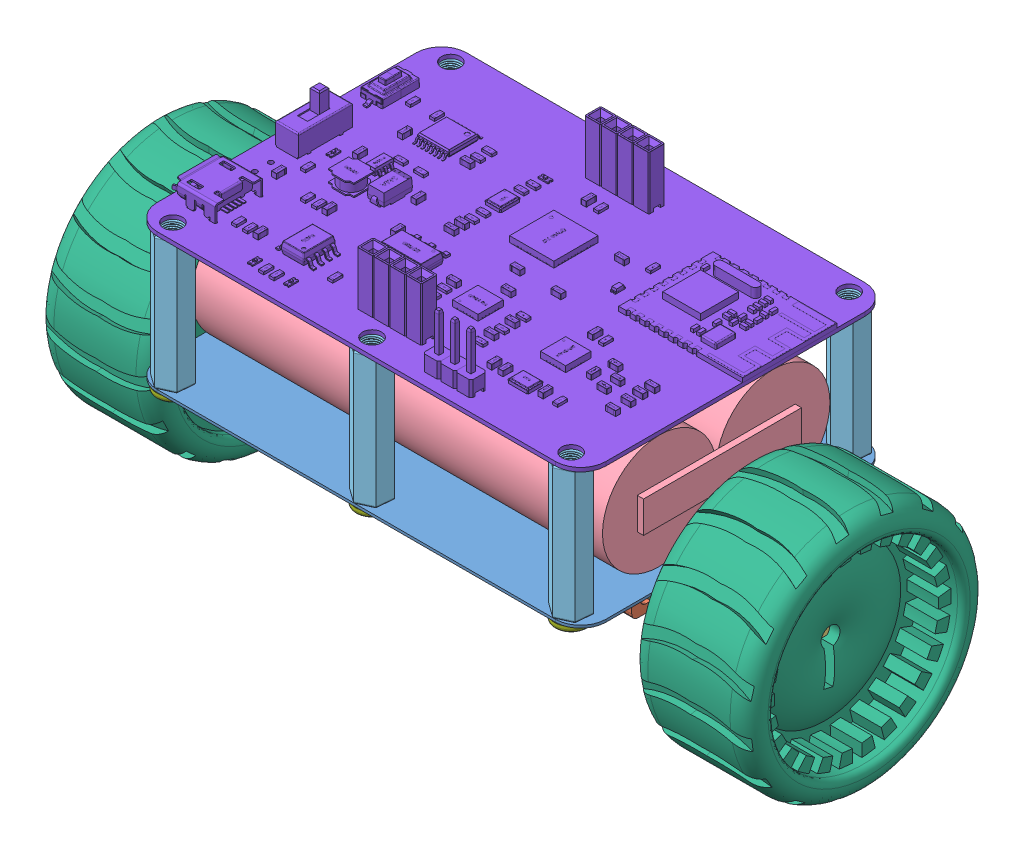
SolidWorks assembly 平衡小车装配体, configuration Default. Lengths in mm.
Overall size (112.99 59.89 50.48).
21 component instances, 8 part files, 29 mates.
Components (placement in the parent):
- 底盘-1: 底盘 [Default] at (53.4104 0 22.4882) x (1 0 -0.000387) z (0 1 0) size (71 49 0.41)
- N20电机座-1: N20电机座 [Default] at (68.1983 -0.4115 22.4825) x (1 0 -0.000387) z (-0.000387 0 -1) size (11.5 11.15 26)
- 电机-1: 电机 [Default] at (68.1983 -5.2615 22.3325) x (0.000387 0 1) z (1 0 -0.000387) size (12.1 14.5 40.5)
- 锂电池-1: 锂电池 [Default] at (20.9104 9 22.5453) x (0.000387 0 1) z (0 1 0) size (36 67 18)
- N20电机座-2: N20电机座 [Default] at (38.6224 -0.4115 22.4939) x (-1 0 0.000387) z (0.000387 0 1) size (11.5 11.15 26)
- 电机-2: 电机 [Default] at (38.6223 -5.2615 22.3439) x (-0.000387 0 -1) z (-1 0 0.000387) size (12.1 14.5 40.5)
- 铜柱M3x21-1: 铜柱M3x21 [Default] at (21.9189 0 44.5004) x (0.910173 0 -0.414228) z (0.414228 0 0.910173) size (5.37 21 4.65)
- 轮子φ43-1: 轮子φ43 [Default] at (100.3983 -5.2615 22.32) x (0.00009 -0.972822 0.231553) z (-0.000376 -0.231553 -0.972822) size (38.37 19 38.37)
- 轮子φ43-2: 轮子φ43 [Default] at (6.4223 -5.2615 22.3564) x (0.00013 -0.942269 0.334857) z (0.000365 0.334857 0.942269) size (38.37 19 38.37)
- 铜柱M3x21-9: 铜柱M3x21 [Default] at (21.9019 0 0.5004) x (0.910173 0 -0.414228) z (0.414228 0 0.910173) size (5.37 21 4.65)
- 铜柱M3x21-10: 铜柱M3x21 [Default] at (53.4189 0 44.4882) x (0.910173 0 -0.414228) z (0.414228 0 0.910173) size (5.37 21 4.65)
- 铜柱M3x21-11: 铜柱M3x21 [Default] at (53.4019 0 0.4882) x (0.910173 0 -0.414228) z (0.414228 0 0.910173) size (5.37 21 4.65)
- 铜柱M3x21-12: 铜柱M3x21 [Default] at (84.9189 0 44.476) x (0.910173 0 -0.414228) z (0.414228 0 0.910173) size (5.37 21 4.65)
- 铜柱M3x21-13: 铜柱M3x21 [Default] at (84.9019 0 0.476) x (0.910173 0 -0.414228) z (0.414228 0 0.910173) size (5.37 21 4.65)
- 螺丝钉M3x6-1: 螺丝钉M3x6 [Default] at (21.9189 -0.4115 44.5004) x (0 1 0) z (0 0 1) size (7.68 5.2 5.2)
- 螺丝钉M3x6-2: 螺丝钉M3x6 [Default] at (21.9019 -0.4115 0.5004) x (0 1 0) z (0 0 1) size (7.68 5.2 5.2)
- 螺丝钉M3x6-3: 螺丝钉M3x6 [Default] at (53.4189 -0.4115 44.4882) x (0 1 0) z (0 0 1) size (7.68 5.2 5.2)
- 螺丝钉M3x6-4: 螺丝钉M3x6 [Default] at (53.4019 -0.4115 0.4882) x (0 1 0) z (0 0 1) size (7.68 5.2 5.2)
- 螺丝钉M3x6-5: 螺丝钉M3x6 [Default] at (84.9189 -0.4115 44.476) x (0 1 0) z (0 0 1) size (7.68 5.2 5.2)
- 螺丝钉M3x6-6: 螺丝钉M3x6 [Default] at (84.9019 -0.4115 0.476) x (0 1 0) z (0 0 1) size (7.68 5.2 5.2)
- 平衡小车主板-1: 平衡小车主板 [Default] at (53.4104 21.6237 22.4882) x (1 0 -0.000387) z (0 1 0) size (71.11 49 13.51)
Mates (geometry in assembly coordinates):
- 重合8: coincident anti-aligned: plane of N20电机座-1 through (79.7006 -0.4115 28.378) normal (-0.000387 0 -1); plane of 电机-1 through (83.2006 -0.2615 28.3767) normal (0.000387 0 1)
- 重合12: coincident anti-aligned: plane of N20电机座-2 through (27.1247 -10.2615 28.3984) normal (-0.000387 0 -1); plane of 电机-2 through (23.6247 -0.2615 28.3997) normal (0.000387 0 1)
- 重合13: coincident anti-aligned: plane of N20电机座-2 through (38.6224 -0.4115 22.4939) normal (1 0 -0.000387); plane of 电机-2 through (38.6223 -5.2615 22.3439) normal (-1 0 0.000387)
- 重合15: coincident aligned: plane of 底盘-1 through (17.9958 0 41.5879) normal (0 1 0)
- 重合17: coincident anti-aligned: plane of 底盘-1 through (22.9017 -0.4115 0) normal (0 0 -1)
- 重合19: coincident anti-aligned: circle of 电机-1; plane of 轮子φ43-1 through (92.8996 -19.8538 25.7962) normal (-1 0 0.000387)
- 同心7: concentric aligned: cylinder of 电机-1 through (102.1983 -5.2615 22.3193) axis (-1 0 0.000387) radius 1.5; cylinder of 轮子φ43-1 through (107.8983 -5.2615 22.3171) axis (-1 0 0.000387) radius 1.5
- 重合20: coincident anti-aligned: plane of 电机-2 through (13.9223 -5.2615 22.3535) normal (-1 0 0.000387); plane of 轮子φ43-2 through (13.9243 -19.3955 27.3763) normal (1 0 -0.000387)
- 同心8: concentric aligned: cylinder of 电机-2 through (4.6223 -5.2615 22.3571) axis (1 0 -0.000387) radius 1.5; cylinder of 轮子φ43-2 through (-1.0777 -5.2615 22.3593) axis (1 0 -0.000387) radius 1.5
- 同心9: concentric anti-aligned: cylinder of N20电机座-2 through (34.407 -1.8115 13.6956) axis (0 1 0) radius 1.125; cylinder of 底盘-1 through (34.407 -0.4115 13.6956) axis (0 -1 0) radius 1.5
- 同心10: concentric anti-aligned: cylinder of 底盘-1 through (34.4138 -0.4115 31.2955) axis (0 -1 0) radius 1.5; cylinder of N20电机座-2 through (34.4138 -1.8115 31.2955) axis (0 1 0) radius 1.125
- 同心11: concentric anti-aligned: cylinder of 底盘-1 through (72.4138 -0.4115 31.2808) axis (0 -1 0) radius 1.5; cylinder of N20电机座-1 through (72.4138 -1.8115 31.2808) axis (0 1 0) radius 1.125
- 同心12: concentric anti-aligned: cylinder of 底盘-1 through (72.407 -0.4115 13.6808) axis (0 -1 0) radius 1.5; cylinder of N20电机座-1 through (72.407 -1.8115 13.6808) axis (0 1 0) radius 1.125
- 重合21: coincident aligned: cylinder of 底盘-1 through (21.9189 -0.4115 44.5004) axis (0 -1 0) radius 1.5; circle of 铜柱M3x21-1
- 重合22: coincident anti-aligned: plane of 底盘-1 through (17.9183 0 43.0149) normal (0 1 0); plane of 铜柱M3x21-1 through (21.9189 0 44.5004) normal (0 -1 0)
- 重合23: coincident anti-aligned: plane of N20电机座-1 through (79.7006 -10.2615 28.378) normal (0 1 0); plane of 电机-1 through (83.1959 -10.2615 16.2767) normal (0 -1 0)
- 重合24: coincident anti-aligned: plane of 底盘-1 through (17.9183 -0.4115 43.0149) normal (0 -1 0); plane of N20电机座-1 through (79.7006 -0.4115 28.378) normal (0 1 0)
- 重合25: coincident anti-aligned: plane of N20电机座-2 through (27.1201 -10.2615 16.5984) normal (0 1 0); plane of 电机-2 through (23.6247 -10.2615 28.3997) normal (0 -1 0)
- 重合26: coincident anti-aligned: plane of 底盘-1 through (17.9183 -0.4115 43.0149) normal (0 -1 0); plane of N20电机座-2 through (27.1201 -0.4115 16.5984) normal (0 1 0)
- 重合27: coincident anti-aligned: plane of N20电机座-1 through (68.1983 -0.4115 22.4825) normal (-1 0 0.000387); plane of 电机-1 through (68.1983 -5.2615 22.3325) normal (1 0 -0.000387)
- 平行1: parallel anti-aligned: plane of 底盘-1 through (17.9183 0 43.0149) normal (0 1 0); plane of 锂电池-1 through (86.9055 6.5 10.0198) normal (0 -1 0)
- 距离1: distance = 6.5 mm anti-aligned: plane of 锂电池-1 through (86.9055 6.5 10.0198) normal (0 -1 0); plane of 底盘-1 through (17.9183 0 43.0149) normal (0 1 0)
- 平行2: parallel aligned: plane of 底盘-1 through (84.8879 -0.4115 -2.024) normal (-0.000387 0 -1); plane of 锂电池-1 through (86.9055 11.5 10.0198) normal (-0.000387 0 -1)
- 距离2: distance = 2 mm aligned: plane of 底盘-1 through (88.9183 -0.4115 42.9875) normal (1 0 -0.000387); plane of 锂电池-1 through (86.9104 9 22.5198) normal (1 0 -0.000387)
- 重合28: coincident anti-aligned: plane of 底盘-1 through (17.9183 -0.4115 43.0149) normal (0 -1 0); plane of 螺丝钉M3x6-1 through (21.9189 -0.4115 44.5004) normal (0 1 0)
- 同心13: concentric aligned: cylinder of 底盘-1 through (21.9189 -0.4115 44.5004) axis (0 -1 0) radius 1.5; circle of 螺丝钉M3x6-1
- 重合29: coincident anti-aligned: plane of 铜柱M3x21-1 through (21.9189 21 44.5004) normal (0 1 0); plane of 平衡小车主板-1 through (17.9183 21 43.0149) normal (0 -1 0)
- 同心14: concentric aligned: cylinder of 铜柱M3x21-1 through (21.9189 21 44.5004) axis (0 -1 0) radius 1.5; cylinder of 平衡小车主板-1 through (21.9189 21 44.5004) axis (0 -1 0) radius 1.5
- 同心15: concentric aligned: cylinder of 铜柱M3x21-13 through (84.9019 21 0.476) axis (0 -1 0) radius 1.5; cylinder of 平衡小车主板-1 through (84.9019 21 0.476) axis (0 -1 0) radius 1.5
